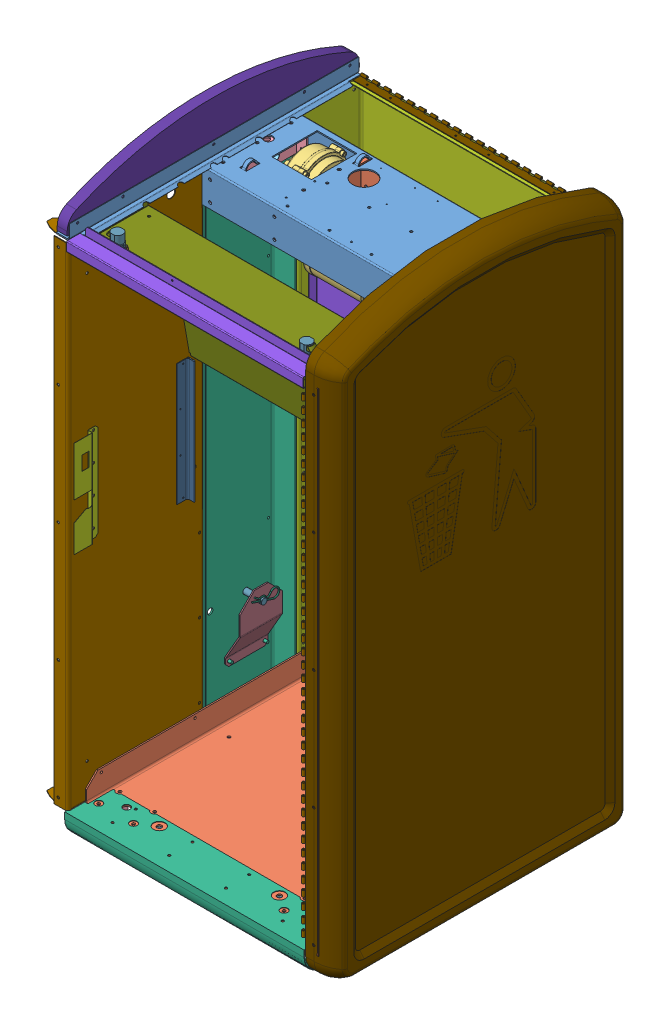
SolidWorks assembly BB3_Chassis, configuration Défaut. Lengths in mm.
Overall size (671.41 1282.03 663.93).
67 component instances, 38 part files, 144 mates.
Components (placement in the parent):
- TopCrossmember_Rev2-1: TopCrossmember_Rev2 [Default] at (20.5473 102.5902 0) size (635 86.99 210.82)
- TopCrossMotorBrkt_Rev3-1: TopCrossMotorBrkt_Rev3 [Défaut] at (-101.9976 61.051 0) size (152.4 200.54 205.51)
- Moto_Reducteur_011_562_1_216-1: Moto_Reducteur_011_562_1_216 [Default] at (192.9322 74.2423 -36.8146) x (0 -0.000019 -1) z (-1 0 0) size (114.3 226.4 239.81)
- TopCrossBearingBrkt_Rev1-1: TopCrossBearingBrkt_Rev1 [Défaut] at (-246.0257 61.051 0) size (25.4 73.66 205.51)
- TopCrossBearingBrkt_Rev1-2: TopCrossBearingBrkt_Rev1 [Défaut] at (287.1203 61.051 0) x (-1 0 0) z (0 0 -1) size (25.4 73.66 205.51)
- Chassis_Coussinet-1: Chassis_Coussinet [Default] at (-247.5497 60.2788 -36.8146) x (0 -0.995993 0.089436) z (0 0.089436 0.995993) size (28.27 19.05 28.27)
- Chassis_Coussinet-2: Chassis_Coussinet [Default] at (288.6443 60.2788 -36.8146) x (0 0.997938 0.064185) z (0 -0.064185 0.997938) size (28.27 19.05 28.27)
- Chassis_Support_Moteur-1: Chassis_Support_Moteur [Défaut] at (-296.9017 100.6288 0.0002) x (0 0 1) z (0 1 0) size (205.51 54 1127)
- Chassis_Support_Moteur-2: Chassis_Support_Moteur [Défaut] at (337.9963 100.6288 0.0002) x (0 0 -1) z (0 1 0) size (205.51 54 1127)
- Chassis_Panneau_Arriere-2: Chassis_Panneau_Arriere [Défaut] at (20.5983 -479.4712 -246.619) x (0 0 1) z (0 1 0) size (164.98 667 1155.29)
- Chassis_Support_Batterie-2: Chassis_Support_Batterie [Défaut] at (20.5983 -270.8192 -242.544) x (0 0 1) z (-1 0 0) size (116.32 446 529)
- Chassis_Support_Moteur_Devant_Gauche-2: Chassis_Support_Moteur_Devant_Gauche [Défaut] at (-249.8894 -442.8187 130.7585) x (0 0 -1) z (0 1 0) size (329.85 66 1105)
- Chassis_Positionnement_Emetteur_Recepteur_Gauche-2: Chassis_Positionnement_Emetteur_Recepteur_Gauche [Défaut] at (-222.4622 -381.8185 156.8606) x (1 0 0) z (0 -1 0) size (22.1 48.5 273)
- Chassis_Support_Moteur_Devant_Droite-1: Chassis_Support_Moteur_Devant_Droite [Défaut] at (290.9839 -442.8187 130.7585) x (0 0 -1) z (0 -1 0) size (329.85 66 1105)
- Chassis_Positionnement_Emetteur_Recepteur_Droite-1: Chassis_Positionnement_Emetteur_Recepteur_Droite [Défaut] at (263.5568 -381.8185 156.8606) x (-1 0 0) z (0 1 0) size (22.1 48.5 273)
- Chassis_Support_Pignon_bas-1: Chassis_Support_Pignon_bas [Défaut] at (305.4963 -865.3715 -39.8528) x (-1 0 0) z (0 0 1) size (35.2 151.29 95)
- Chassis_Axe_Pignon_Bas-1: Chassis_Axe_Pignon_Bas [Défaut] at (340.9963 -816.3715 -39.8528) x (-1 0 0) z (0 -0.052233 -0.998635) size (48.6 15.9 15.9)
- Chassis_Goupille_Axe_Pignon_bas-1: Chassis_Goupille_Axe_Pignon_bas [Défaut] at (300.5463 -817.6251 -63.8201) x (0 0.052233 0.998635) z (1 0 0) size (60.5 23 3)
- Chassis_Support_Pignon_bas-2: Chassis_Support_Pignon_bas [Défaut] at (-264.4017 -865.3715 -39.8528) x (1 0 0) z (0 0 -1) size (35.2 151.29 95)
- Chassis_Axe_Pignon_Bas-2: Chassis_Axe_Pignon_Bas [Défaut] at (-299.9017 -816.3715 -39.8528) x (1 0 0) z (0 0.31653 0.948583) size (48.6 15.9 15.9)
- Chassis_Goupille_Axe_Pignon_bas-2: Chassis_Goupille_Axe_Pignon_bas [Défaut] at (-259.4517 -808.7748 -17.0869) x (0 -0.31653 -0.948583) z (1 0 0) size (60.5 23 3)
- Chassis_Plaque_Haute-1: Chassis_Plaque_Haute [Défaut] at (20.4963 92.768 412.6062) x (0 0 -1) z (1 0 0) size (278.51 354.1 562.7)
- Chassis_Renfort-1: Chassis_Renfort [Défaut] at (20.5463 -1018.8712 0.0002) x (0 0 1) z (-1 0 0) size (199.51 39 641)
- Chassis_Charniere_Photovoltaique-1: Chassis_Charniere_Photovoltaique [Défaut] at (20.5983 134.4053 -220.1468) x (0 0 -1) z (1 0 0) size (21.77 6 520)
- Chassis_Equerre_Haute-1: Chassis_Equerre_Haute [Défaut] at (-246.1446 112.2812 81.6782) x (1 0 0.000001) z (-0.000001 0 1) size (44 37.45 648)
- Chassis_Equerre_Haute-2: Chassis_Equerre_Haute [Défaut] at (287.2893 112.2812 81.6751) x (-1 0 -0.000168) z (0.000168 0 -1) size (44 37.45 648)
- Chassis_Repose_Bac_Dechets-1: Chassis_Repose_Bac_Dechets [Défaut] at (20.4963 -992.8728 80.2436) x (0 -0.000001 1) z (-1 0 0) size (641.73 77 529)
- Chassis_Semelle-1: Chassis_Semelle [Défaut] at (20.4963 -1034.3925 80.4561) x (1 0 0) z (0 -0.000001 1) size (404.15 56 558)
- Chassis_Repose_Pied-1: Chassis_Repose_Pied [Défaut] at (-187.0037 -1049.3185 336.4561) x (1 0 0) z (0 -0.000001 1) size (94 52.5 63.3)
- Chassis_Repose_Pied-2: Chassis_Repose_Pied [Défaut] at (-187.0037 -1049.3182 -175.5439) x (1 0 0) z (0 -0.000001 1) size (94 52.5 63.3)
- Chassis_Repose_Pied-3: Chassis_Repose_Pied [Défaut] at (227.9963 -1049.3182 -175.5439) x (1 0 0) z (0 -0.000001 1) size (94 52.5 63.3)
- Chassis_Repose_Pied-4: Chassis_Repose_Pied [Défaut] at (227.9963 -1049.3185 336.4561) x (1 0 0) z (0 -0.000001 1) size (94 52.5 63.3)
- Chassis_Repose_Pied_Insert-1: Chassis_Repose_Pied_Insert [Défaut] at (-187.0037 -1050.3185 336.4561) x (0 1 0.000001) z (0.428959 -0.000001 0.903324) size (14.3 17.5 17.5)
- Chassis_Repose_Pied_Insert-2: Chassis_Repose_Pied_Insert [Défaut] at (227.9963 -1050.3185 336.4561) x (0 1 0.000001) z (0.384049 -0.000001 0.923313) size (14.3 17.5 17.5)
- Chassis_Repose_Pied_Insert-3: Chassis_Repose_Pied_Insert [Défaut] at (227.9963 -1050.3182 -175.5439) x (0 1 0.000001) z (-0.000001 -0.000001 1) size (14.3 17.5 17.5)
- Chassis_Repose_Pied_Insert-4: Chassis_Repose_Pied_Insert [Défaut] at (-187.0037 -1050.3182 -175.5439) x (0 1 0.000001) z (-0.000001 -0.000001 1) size (14.3 17.5 17.5)
- Chassis_Repose_Pied_Insert-5: Chassis_Repose_Pied_Insert [Défaut] at (-114.0037 -995.8185 336.4561) x (0 -1 -0.000001) z (0.798225 0 0.602359) size (14.3 17.5 17.5)
- Chassis_Repose_Pied_Insert-6: Chassis_Repose_Pied_Insert [Défaut] at (154.9963 -995.8185 336.4561) x (0 -1 -0.000001) z (0.000001 -0.000001 1) size (14.3 17.5 17.5)
- Chassis_Repose_Pied_Insert-7: Chassis_Repose_Pied_Insert [Défaut] at (-114.0037 -995.8182 -175.5439) x (0 -1 -0.000001) z (0.000001 -0.000001 1) size (14.3 17.5 17.5)
- Chassis_Repose_Pied_Insert-8: Chassis_Repose_Pied_Insert [Défaut] at (154.9963 -995.8182 -175.5439) x (0 -1 -0.000001) z (0.000001 -0.000001 1) size (14.3 17.5 17.5)
- Chassis_Dessous_Avant_Porte-1: Chassis_Dessous_Avant_Porte [Défaut] at (20.4963 -992.8728 80.2436) x (0 -0.000001 1) z (-1 0 0) size (98 53.79 536)
- Chassis_Serrure-1: Chassis_Serrure [Défaut] at (-243.4017 -382.964 366.4072) x (1 0 0) z (0 1 0) size (10.5 63.82 216)
- Chassis_Equerre_Face-1: Chassis_Equerre_Face [Défaut] at (20.4963 111.0096 411.9878) x (0 0 1) z (-1 0 0) size (32.2 41.42 529)
- Chassis_Charniere_Support_Moteur_Devant_Droite-1: Chassis_Charniere_Support_Moteur_Devant_Droite [Défaut] at (260.2718 -465.3185 388.412) x (0 0 1) z (0 -1 0) size (21.77 6 1066)
- Chassis_Serrure_Cle-1: Chassis_Serrure_Cle [Défaut] at (-191.3537 126.1269 363.7894) x (0 1 0) z (-1 0 0) size (41.58 38.56 38.97)
  - Chassis_Serrure_Came-1: Chassis_Serrure_Came [Défaut] at (-18.246 14.5659 16.3878) x (0 -1 0) z (1 0 0) size (12.45 12.01 13.54)
  - Chassis_Serrure_Rondelle_Ecrou-1: Chassis_Serrure_Rondelle_Ecrou [Défaut] at (-31.074 17.7899 -9.8703) x (0 0.096744 0.995309) z (-1 0 0) size (35.31 35.31 0.64)
  - Chassis_Serrure_Ecrou_Hex-1: Chassis_Serrure_Ecrou_Hex [Défaut] at (-26.3115 -31.157 8.2014) x (0 0 1) z (-1 0 0) size (33 28.58 4.76)
  - Chassis_Serrure_Insert_Cle-1: Chassis_Serrure_Insert_Cle [Défaut] at (26.379 -212.8643 14.6) x (-1 0 0) z (0 0 -1) size (23.33 15.95 15.95)
  - Chassis_Serrure_Support-1: Chassis_Serrure_Support [Défaut] at (-26.6815 11.1833 12.473) x (-1 0 0) z (0 -1 0) size (41.46 28.7 28.7)
  - Chassis_Serrure_Ressort-1: Chassis_Serrure_Ressort [Défaut] at (-1.4058 10.243 9.1044) x (0 0 -1) z (1 0 0) size (21.49 4.59 4.57)
  - Chassis_Serrure_Pene-1: Chassis_Serrure_Pene [Défaut] at (1.0072 5.2825 -10.1896) x (0 -0.999973 -0.007317) z (-1 0 0) size (16.91 23.47 9.63)
- Chassis_Serrure_Cle-2: Chassis_Serrure_Cle [Défaut] at (232.3463 126.1269 341.4229) x (0 1 0) z (1 0 0) size (41.58 38.56 38.97)
  - Chassis_Serrure_Came-1: Chassis_Serrure_Came [Défaut] at (-18.246 14.5659 16.3878) x (0 -1 0) z (1 0 0) size (12.45 12.01 13.54)
  - Chassis_Serrure_Rondelle_Ecrou-1: Chassis_Serrure_Rondelle_Ecrou [Défaut] at (-31.074 17.7899 -9.8703) x (0 0.096744 0.995309) z (-1 0 0) size (35.31 35.31 0.64)
  - Chassis_Serrure_Ecrou_Hex-1: Chassis_Serrure_Ecrou_Hex [Défaut] at (-26.3115 -31.157 8.2014) x (0 0 1) z (-1 0 0) size (33 28.58 4.76)
  - Chassis_Serrure_Insert_Cle-1: Chassis_Serrure_Insert_Cle [Défaut] at (26.379 -212.8643 14.6) x (-1 0 0) z (0 0 -1) size (23.33 15.95 15.95)
  - Chassis_Serrure_Support-1: Chassis_Serrure_Support [Défaut] at (-26.6815 11.1833 12.473) x (-1 0 0) z (0 -1 0) size (41.46 28.7 28.7)
  - Chassis_Serrure_Ressort-1: Chassis_Serrure_Ressort [Défaut] at (-1.4058 10.243 9.1044) x (0 0 -1) z (1 0 0) size (21.49 4.59 4.57)
  - Chassis_Serrure_Pene-1: Chassis_Serrure_Pene [Défaut] at (1.0072 5.2825 -10.1896) x (0 -0.999973 -0.007317) z (-1 0 0) size (16.91 23.47 9.63)
- Tombstone_Rev1-1: Tombstone_Rev1 [Default] at (288.5894 129.5652 81.0473) x (1 0 0.000168) z (-0.000168 0 1) size (22.23 105.62 654.05)
- Tombstone_Rev1-2: Tombstone_Rev1 [Default] at (-247.4446 129.5652 82.3062) x (-1 0 -0.000001) z (0.000001 0 -1) size (22.23 105.62 654.05)
- SideSkin_Rev1-1: SideSkin_Rev1 [Default] at (-317.3073 -1045.6118 82.3061) x (-1 0 -0.000001) z (0.000001 0 -1) size (69.87 1274.83 660.4) (hidden)
- SideSkin_Rev1-2: SideSkin_Rev1 [Default] at (358.4521 -1045.6118 81.059) x (1 0 0.000168) z (-0.000168 0 1) size (69.87 1274.83 660.4)
- Chassis_Interieur_Cache_Chaine-1: Chassis_Interieur_Cache_Chaine [Défaut] at (-242.9017 -763.8184 0) x (0 -0.000001 1) z (-1 0 0) size (249 989 21) (hidden)
- Chassis_Interieur_Cache_Chaine-2: Chassis_Interieur_Cache_Chaine [Défaut] at (283.9963 -763.8185 0.0002) x (0 0 -1) z (1 0 0) size (249 989 21)
- Chassis_Bac_Dechets-1: Chassis_Bac_Dechets [Défaut] at (19.5983 -711.9931 65.1059) x (-1 0 0) z (0 0.000001 -1) size (517 387.96 620.45) (hidden)
Mates (geometry in assembly coordinates):
- Coïncidente2: coincident anti-aligned: plane of TopCrossmember_Rev2-1 through (338.0473 102.5902 -102.7532) normal (0 0 1); plane of TopCrossMotorBrkt_Rev3-1 through (50.4024 28.92 -102.7532) normal (0 0 -1)
- Coaxiale4: concentric aligned: cylinder of TopCrossmember_Rev2-1 through (-87.4027 86.197 105.41) axis (0 0 1) radius 3.3735; cylinder of TopCrossMotorBrkt_Rev3-1 through (-87.4027 86.197 102.7532) axis (0 0 1) radius 3.3735
- Coaxiale5: concentric aligned: cylinder of TopCrossmember_Rev2-1 through (-87.4027 41.747 105.41) axis (0 0 1) radius 3.3735; cylinder of TopCrossMotorBrkt_Rev3-1 through (-87.4027 41.747 102.7532) axis (0 0 1) radius 3.3735
- Coïncidente3: coincident anti-aligned: plane of TopCrossMotorBrkt_Rev3-1 through (-101.9976 19.522 -102.7532) normal (-1 0 0); plane of Moto_Reducteur_011_562_1_216-1 through (-101.9976 60.2791 -36.8143) normal (1 0 0)
- Coaxiale6: concentric anti-aligned: cylinder of TopCrossMotorBrkt_Rev3-1 through (-99.3407 60.2788 -36.8146) axis (-1 0 0) radius 15.24; cylinder of Moto_Reducteur_011_562_1_216-1 through (-181.2456 60.2791 -36.8143) axis (1 0 0) radius 9.525
- Coaxiale7: concentric anti-aligned: cylinder of TopCrossMotorBrkt_Rev3-1 through (-99.3407 33.3368 -63.7556) axis (-1 0 0) radius 3.683; cylinder of Moto_Reducteur_011_562_1_216-1 through (-101.9976 33.3368 -63.7556) axis (1 0 0) radius 3.175
- Coïncidente4: coincident anti-aligned: plane of TopCrossmember_Rev2-1 through (-296.9527 102.5902 102.7532) normal (0 0 -1); plane of TopCrossBearingBrkt_Rev1-1 through (-243.3689 94.96 102.7532) normal (0 0 1)
- Coaxiale8: concentric aligned: cylinder of TopCrossmember_Rev2-1 through (-231.4207 86.197 105.41) axis (0 0 1) radius 3.3735; cylinder of TopCrossBearingBrkt_Rev1-1 through (-231.4207 86.197 102.7532) axis (0 0 1) radius 3.3735
- Coaxiale9: concentric aligned: cylinder of TopCrossmember_Rev2-1 through (-231.4207 41.747 105.41) axis (0 0 1) radius 3.3735; cylinder of TopCrossBearingBrkt_Rev1-1 through (-231.4207 41.747 102.7532) axis (0 0 1) radius 3.3735
- Coïncidente5: coincident anti-aligned: plane of TopCrossmember_Rev2-1 through (338.0473 102.5902 -102.7532) normal (0 0 1); plane of TopCrossBearingBrkt_Rev1-2 through (284.4634 94.96 -102.7532) normal (0 0 -1)
- Coaxiale10: concentric anti-aligned: cylinder of TopCrossmember_Rev2-1 through (272.5153 86.197 105.41) axis (0 0 1) radius 3.3735; cylinder of TopCrossBearingBrkt_Rev1-2 through (272.5153 86.197 -102.7532) axis (0 0 -1) radius 3.3735
- Coaxiale11: concentric anti-aligned: cylinder of TopCrossmember_Rev2-1 through (272.5153 41.747 105.41) axis (0 0 1) radius 3.3735; cylinder of TopCrossBearingBrkt_Rev1-2 through (272.5153 41.747 -102.7532) axis (0 0 -1) radius 3.3735
- Coïncidente6: coincident anti-aligned: plane of TopCrossBearingBrkt_Rev1-1 through (-246.0257 19.522 -102.7532) normal (-1 0 0); plane of Chassis_Coussinet-1 through (-246.0257 60.2788 -36.8146) normal (1 0 0)
- Coaxiale12: concentric anti-aligned: cylinder of TopCrossBearingBrkt_Rev1-1 through (-243.3689 60.2788 -36.8146) axis (-1 0 0) radius 11.1125; cylinder of Chassis_Coussinet-1 through (-247.5497 60.2788 -36.8146) axis (1 0 0) radius 9.6139
- Coaxiale13: concentric anti-aligned: cylinder of TopCrossBearingBrkt_Rev1-2 through (284.4634 60.2788 -36.8146) axis (1 0 0) radius 11.1125; cylinder of Chassis_Coussinet-2 through (269.5943 60.2788 -36.8146) axis (-1 0 0) radius 11.1125
- Coïncidente7: coincident anti-aligned: plane of TopCrossBearingBrkt_Rev1-2 through (287.1203 19.522 102.7532) normal (1 0 0); plane of Chassis_Coussinet-2 through (287.1203 60.2788 -36.8146) normal (-1 0 0)
- Coïncidente8: coincident anti-aligned: plane of TopCrossmember_Rev2-1 through (-269.9017 102.5902 0) normal (-1 0 0); plane of Chassis_Support_Moteur-1
- Coïncidente12: coincident anti-aligned: plane of TopCrossmember_Rev2-1 through (-296.9527 102.5902 102.7532) normal (0 0 -1); plane of Chassis_Support_Moteur-1 through (-299.9017 100.6288 102.7532) normal (0 0 1)
- Coïncidente13: coincident anti-aligned: plane of TopCrossBearingBrkt_Rev1-1 through (-246.0257 60.2788 0) normal (0 1 0); plane of Chassis_Support_Moteur-1
- Coïncidente14: coincident anti-aligned: plane of TopCrossmember_Rev2-1 through (-296.9527 102.5902 102.7532) normal (0 0 -1); plane of Chassis_Support_Moteur-2 through (286.9963 100.6288 102.7532) normal (0 0 1)
- Coïncidente15: coincident anti-aligned: plane of TopCrossBearingBrkt_Rev1-2; plane of Chassis_Support_Moteur-2
- Coïncidente16: coincident anti-aligned: plane of TopCrossmember_Rev2-1 through (310.9963 102.5902 0) normal (1 0 0); plane of Chassis_Support_Moteur-2
- Coaxiale15: concentric aligned: cylinder of Chassis_Support_Moteur-1 through (-298.4017 10.6288 -90.7528) axis (1 0 0) radius 2.45; cylinder of Chassis_Panneau_Arriere-2 through (-301.4017 10.6288 -90.7528) axis (1 0 0) radius 2.7
- Coaxiale16: concentric aligned: cylinder of Chassis_Support_Moteur-1 through (-298.4017 -903.3712 -90.7528) axis (1 0 0) radius 2.45; cylinder of Chassis_Panneau_Arriere-2 through (-301.4017 -903.3712 -90.7528) axis (1 0 0) radius 2.7
- Coïncidente19: coincident anti-aligned: plane of Chassis_Support_Moteur-1 through (-299.9017 100.6288 0.0002) normal (-1 0 0); plane of Chassis_Panneau_Arriere-2 through (-299.9017 -1095.4712 -106.044) normal (1 0 0)
- Coïncidente20: coincident anti-aligned: plane of Chassis_Panneau_Arriere-2 through (285.0983 -998.3712 -112.044) normal (-1 0 0); plane of Chassis_Support_Batterie-2 through (285.0983 -476.3192 -146.144) normal (1 0 0)
- Coaxiale17: concentric aligned: cylinder of Chassis_Panneau_Arriere-2 through (285.8483 -484.8192 -214.144) axis (-1 0 0) radius 2.7; cylinder of Chassis_Support_Batterie-2 through (285.0983 -484.8192 -214.144) axis (-1 0 0) radius 2.7
- Coaxiale18: concentric aligned: cylinder of Chassis_Panneau_Arriere-2 through (285.8483 -484.8192 -158.144) axis (-1 0 0) radius 2.7; cylinder of Chassis_Support_Batterie-2 through (285.0983 -484.8192 -158.144) axis (-1 0 0) radius 2.7
- Coaxiale19: concentric aligned: cylinder of Chassis_Support_Moteur-1 through (-299.9017 10.6288 90.7532) axis (1 0 0) radius 2.45; cylinder of Chassis_Support_Moteur_Devant_Gauche-2 through (-301.4017 10.6288 90.7532) axis (1 0 0) radius 2.7
- Coaxiale20: concentric aligned: cylinder of Chassis_Support_Moteur-1 through (-299.9017 -903.3712 90.7532) axis (1 0 0) radius 2.45; cylinder of Chassis_Support_Moteur_Devant_Gauche-2 through (-301.4017 -903.3712 90.7532) axis (1 0 0) radius 2.7
- Coïncidente21: coincident anti-aligned: plane of Chassis_Support_Moteur-1 through (-299.9017 100.6288 0.0002) normal (-1 0 0); plane of Chassis_Support_Moteur_Devant_Gauche-2 through (-299.9017 -1056.8712 80.7532) normal (1 0 0)
- Coïncidente22: coincident anti-aligned: plane of Chassis_Support_Moteur_Devant_Gauche-2 through (-243.9017 -1056.8712 104.9532) normal (1 0 0); plane of Chassis_Positionnement_Emetteur_Recepteur_Gauche-2 through (-243.9017 -245.3185 143.1532) normal (-1 0 0)
- Coaxiale21: concentric aligned: cylinder of Chassis_Support_Moteur_Devant_Gauche-2 through (-245.4017 -426.8185 160.4532) axis (1 0 0) radius 1.5; cylinder of Chassis_Positionnement_Emetteur_Recepteur_Gauche-2 through (-243.9017 -426.8185 160.4532) axis (1 0 0) radius 1.5
- Coaxiale22: concentric aligned: cylinder of Chassis_Support_Moteur_Devant_Gauche-2 through (-245.4017 -336.8185 160.4532) axis (1 0 0) radius 1.5; cylinder of Chassis_Positionnement_Emetteur_Recepteur_Gauche-2 through (-243.9017 -336.8185 160.4532) axis (1 0 0) radius 1.5
- Coïncidente24: coincident anti-aligned: plane of Chassis_Support_Moteur-2 through (340.9963 100.6288 0.0002) normal (1 0 0); plane of Chassis_Support_Moteur_Devant_Droite-1 through (340.9963 27.0338 80.7532) normal (-1 0 0)
- Coaxiale25: concentric aligned: cylinder of Chassis_Support_Moteur-2 through (339.4963 10.6288 90.7532) axis (-1 0 0) radius 2.45; cylinder of Chassis_Support_Moteur_Devant_Droite-1 through (341.7463 10.6288 90.7532) axis (-1 0 0) radius 2.7
- Coaxiale26: concentric aligned: cylinder of Chassis_Support_Moteur-2 through (339.4963 -903.3712 90.7532) axis (-1 0 0) radius 2.45; cylinder of Chassis_Support_Moteur_Devant_Droite-1 through (341.7463 -903.3712 90.7532) axis (-1 0 0) radius 2.7
- Coïncidente26: coincident anti-aligned: plane of Chassis_Support_Moteur_Devant_Droite-1 through (284.9963 103.6812 110.9532) normal (-1 0 0); plane of Chassis_Positionnement_Emetteur_Recepteur_Droite-1 through (284.9963 -245.3185 168.4532) normal (1 0 0)
- Coaxiale27: concentric aligned: cylinder of Chassis_Support_Moteur_Devant_Droite-1 through (285.7463 -336.8185 160.4532) axis (-1 0 0) radius 1.5; cylinder of Chassis_Positionnement_Emetteur_Recepteur_Droite-1 through (284.3463 -336.8185 160.4532) axis (-1 0 0) radius 1.5
- Coaxiale28: concentric aligned: cylinder of Chassis_Support_Moteur_Devant_Droite-1 through (285.7463 -426.8185 160.4532) axis (-1 0 0) radius 1.5; cylinder of Chassis_Positionnement_Emetteur_Recepteur_Droite-1 through (284.3463 -426.8185 160.4532) axis (-1 0 0) radius 1.5
- Coïncidente27: coincident anti-aligned: plane of Chassis_Support_Moteur-2 through (337.9963 100.6288 -99.7528) normal (-1 0 0); plane of Chassis_Support_Pignon_bas-1 through (337.9963 -921.6632 -87.3528) normal (1 0 0)
- Coaxiale29: concentric aligned: cylinder of Chassis_Support_Moteur-2 through (340.9963 -930.8712 -79.7058) axis (-1 0 0) radius 3; cylinder of Chassis_Support_Pignon_bas-1 through (337.9963 -930.8712 -79.7058) axis (-1 0 0) radius 3.5
- Coaxiale30: concentric aligned: cylinder of Chassis_Support_Moteur-2 through (340.9963 -930.8712 0.0002) axis (-1 0 0) radius 3; cylinder of Chassis_Support_Pignon_bas-1 through (337.9963 -930.8712 0.0002) axis (-1 0 0) radius 3.5
- Coïncidente28: coincident anti-aligned: plane of Chassis_Support_Moteur-2 through (340.9963 100.6288 0.0002) normal (1 0 0); plane of Chassis_Axe_Pignon_Bas-1 through (340.9963 -812.4019 -40.0605) normal (-1 0 0)
- Coaxiale31: concentric anti-aligned: cylinder of Chassis_Support_Pignon_bas-1 through (302.7963 -816.3715 -39.8528) axis (1 0 0) radius 6.5; cylinder of Chassis_Axe_Pignon_Bas-1 through (318.6963 -816.3715 -39.8528) axis (-1 0 0) radius 6.25
- Coaxiale32: concentric anti-aligned: cylinder of Chassis_Axe_Pignon_Bas-1 through (300.5463 -819.1686 -93.3295) axis (0 -0.052233 -0.998635) radius 2.15; cylinder of Chassis_Goupille_Axe_Pignon_bas-1 through (300.5463 -817.6251 -63.8201) axis (0 0.052233 0.998635) radius 1.5
- Parallèle1: parallel anti-aligned: plane of Chassis_Support_Pignon_bas-1 through (302.7963 -866.095 -87.3528) normal (-1 0 0); plane of Chassis_Goupille_Axe_Pignon_bas-1 through (300.5463 -817.6251 -63.8201) normal (1 0 0)
- Tangent2: tangent: cylinder of Chassis_Axe_Pignon_Bas-1 through (318.6963 -816.3715 -39.8528) axis (-1 0 0) radius 6.25; face of Chassis_Goupille_Axe_Pignon_bas-1
- Coïncidente29: coincident anti-aligned: plane of Chassis_Support_Moteur-1 through (-296.9017 100.6288 99.7532) normal (1 0 0); plane of Chassis_Support_Pignon_bas-2 through (-296.9017 -913.016 6.2972) normal (-1 0 0)
- Coaxiale33: concentric aligned: cylinder of Chassis_Support_Moteur-1 through (-296.9017 -930.8712 -79.7058) axis (1 0 0) radius 3; cylinder of Chassis_Support_Pignon_bas-2 through (-296.9017 -930.8712 -79.7058) axis (1 0 0) radius 3.5
- Coïncidente30: coincident anti-aligned: plane of Chassis_Support_Moteur-1 through (-299.9017 100.6288 0.0002) normal (-1 0 0); plane of Chassis_Axe_Pignon_Bas-2 through (-299.9017 -809.2033 -52.7033) normal (1 0 0)
- Coaxiale35: concentric anti-aligned: cylinder of Chassis_Support_Pignon_bas-2 through (-261.7017 -812.9739 -51.4451) axis (-1 0 0) radius 6.5; cylinder of Chassis_Axe_Pignon_Bas-2 through (-277.6017 -812.9739 -51.4451) axis (1 0 0) radius 6.25
- Coaxiale36: concentric anti-aligned: cylinder of Chassis_Axe_Pignon_Bas-2 through (-259.4517 -796.0238 -0.6487) axis (0 0.31653 0.948583) radius 2.15; cylinder of Chassis_Goupille_Axe_Pignon_bas-2 through (-259.4517 -805.3772 -28.6791) axis (0 -0.31653 -0.948583) radius 1.5
- Parallèle2: parallel aligned: plane of Chassis_Support_Pignon_bas-2 through (-261.7017 -857.7236 0.7674) normal (1 0 0); plane of Chassis_Goupille_Axe_Pignon_bas-2 through (-259.4517 -805.3772 -28.6791) normal (1 0 0)
- Tangent3: tangent: cylinder of Chassis_Axe_Pignon_Bas-2 through (-277.6017 -812.9739 -51.4451) axis (1 0 0) radius 6.25; face of Chassis_Goupille_Axe_Pignon_bas-2
- Coaxiale39: concentric aligned: cylinder of Chassis_Support_Moteur_Devant_Droite-1 through (285.7463 99.9922 260.6062) axis (-1 0 0) radius 2.7; cylinder of Chassis_Plaque_Haute-1 through (284.1713 99.9922 260.6062) axis (-1 0 0) radius 2.7
- Coaxiale40: concentric aligned: cylinder of Chassis_Support_Moteur_Devant_Droite-1 through (285.7463 99.9922 387.6062) axis (-1 0 0) radius 2.7; cylinder of Chassis_Plaque_Haute-1 through (284.1713 99.9922 387.6062) axis (-1 0 0) radius 2.7
- Coïncidente32: coincident anti-aligned: plane of Chassis_Support_Moteur_Devant_Droite-1 through (284.9963 103.6812 110.9532) normal (-1 0 0); plane of Chassis_Plaque_Haute-1 through (284.9963 -169.3578 412.6062) normal (1 0 0)
- Coaxiale41: concentric anti-aligned: cylinder of Chassis_Support_Moteur-2 through (314.9963 -1012.3712 -102.7528) axis (0 0 1) radius 5; cylinder of Chassis_Renfort-1 through (314.9963 -1012.3712 -96.7528) axis (0 0 -1) radius 4.25
- Coïncidente33: coincident anti-aligned: plane of Chassis_Support_Moteur-2 through (286.9963 100.6288 -99.7528) normal (0 0 1); plane of Chassis_Renfort-1 through (341.0463 -1038.3712 -99.7528) normal (0 0 -1)
- Angle1: planar angle = 0 rad aligned: plane of Chassis_Support_Moteur-2 through (330.2237 -1026.3712 -67.6038) normal (0 -1 0); plane of Chassis_Renfort-1 through (341.0463 -1002.3712 96.7532) normal (0 -1 0)
- Coïncidente34: coincident anti-aligned: plane of Chassis_Panneau_Arriere-2 through (-245.4017 109.6808 -1447.8763) normal (0 1 0); plane of Chassis_Charniere_Photovoltaique-1 through (20.5983 109.6808 -241.391) normal (0 -1 0)
- Coaxiale42: concentric anti-aligned: cylinder of Chassis_Panneau_Arriere-2 through (255.5983 109.6808 -229.619) axis (0 -1 0) radius 2.7; cylinder of Chassis_Charniere_Photovoltaique-1 through (255.5983 109.6808 -229.619) axis (0 1 0) radius 1.75
- Coaxiale43: concentric anti-aligned: cylinder of Chassis_Panneau_Arriere-2 through (-214.4017 109.6808 -229.619) axis (0 -1 0) radius 2.7; cylinder of Chassis_Charniere_Photovoltaique-1 through (-214.4017 109.6808 -229.619) axis (0 1 0) radius 1.75
- Coïncidente35: coincident anti-aligned: plane of Chassis_Support_Moteur_Devant_Gauche-2 through (918.7559 109.6812 104.9532) normal (0 1 0); plane of Chassis_Equerre_Haute-1 through (-241.0792 109.6812 81.6782) normal (0 -1 0)
- Coaxiale46: concentric anti-aligned: cylinder of Chassis_Support_Moteur_Devant_Gauche-2 through (-264.6447 108.9312 379.9532) axis (0 -1 0) radius 2.7; cylinder of Chassis_Equerre_Haute-1 through (-264.6447 110.9812 379.9532) axis (0 1 0) radius 2.85
- Coaxiale47: concentric anti-aligned: cylinder of Chassis_Panneau_Arriere-2 through (-264.6444 109.6808 -226.322) axis (0 -1 0) radius 2.6; cylinder of Chassis_Equerre_Haute-1 through (-264.6444 110.9812 -226.3218) axis (0 1 0) radius 2.85
- Coïncidente38: coincident anti-aligned: plane of Chassis_Support_Moteur_Devant_Droite-1 through (350.9966 109.6812 110.9532) normal (0 1 0); plane of Chassis_Equerre_Haute-2 through (282.224 109.6812 81.6742) normal (0 -1 0)
- Coaxiale48: concentric anti-aligned: cylinder of Chassis_Support_Moteur_Devant_Droite-1 through (305.7393 109.6812 379.9532) axis (0 -1 0) radius 2.7; cylinder of Chassis_Equerre_Haute-2 through (305.7393 110.9812 379.9532) axis (0 1 0) radius 2.85
- Coaxiale49: concentric anti-aligned: cylinder of Chassis_Panneau_Arriere-2 through (305.841 108.9308 -226.322) axis (0 -1 0) radius 2.6; cylinder of Chassis_Equerre_Haute-2 through (305.841 110.9812 -226.3218) axis (0 1 0) radius 2.85
- Coaxiale50: concentric aligned: cylinder of Chassis_Panneau_Arriere-2 through (285.8483 -950.8182 -172.627) axis (-1 0 0) radius 2.7; cylinder of Chassis_Repose_Bac_Dechets-1 through (284.9963 -950.8182 -172.6268) axis (-1 0 0) radius 2.7
- Coaxiale51: concentric aligned: cylinder of Chassis_Support_Moteur_Devant_Droite-1 through (285.7463 -950.8185 339.1062) axis (-1 0 0) radius 2.7; cylinder of Chassis_Repose_Bac_Dechets-1 through (284.9963 -950.8185 339.1062) axis (-1 0 0) radius 2.7
- Coïncidente39: coincident anti-aligned: plane of Chassis_Support_Moteur_Devant_Droite-1 through (284.9963 103.6812 110.9532) normal (-1 0 0); plane of Chassis_Repose_Bac_Dechets-1 through (284.9963 -968.3183 80.2436) normal (1 0 0)
- Coïncidente40: coincident anti-aligned: plane of Chassis_Repose_Bac_Dechets-1 through (284.9963 -996.8185 398.1061) normal (0 -1 -0.000001); plane of Chassis_Semelle-1 through (-128.6584 -996.8181 -198.5439) normal (0 1 0.000001)
- Coaxiale53: concentric aligned: cylinder of Chassis_Repose_Bac_Dechets-1 through (-114.0037 -993.8185 336.4561) axis (0 -1 -0.000001) radius 5.25; cylinder of Chassis_Semelle-1 through (-114.0037 -996.8185 336.4561) axis (0 -1 -0.000001) radius 6.75
- Coaxiale54: concentric aligned: cylinder of Chassis_Repose_Bac_Dechets-1 through (-114.0037 -993.8182 -175.5439) axis (0 -1 -0.000001) radius 5.25; cylinder of Chassis_Semelle-1 through (-114.0037 -996.8182 -175.5439) axis (0 -1 -0.000001) radius 6.75
- Coïncidente41: coincident anti-aligned: plane of Chassis_Repose_Bac_Dechets-1 through (284.9963 -996.8185 398.1061) normal (0 -1 -0.000001); plane of Chassis_Repose_Pied-1 through (-234.0037 -996.8185 304.8061) normal (0 1 0.000001)
- Coaxiale55: concentric aligned: cylinder of Chassis_Repose_Bac_Dechets-1 through (-226.0037 -993.8185 312.8061) axis (0 -1 -0.000001) radius 3.25; cylinder of Chassis_Repose_Pied-1 through (-226.0037 -996.8185 312.8061) axis (0 -1 -0.000001) radius 3.25
- Coaxiale56: concentric aligned: cylinder of Chassis_Repose_Bac_Dechets-1 through (-226.0037 -993.8185 360.1061) axis (0 -1 -0.000001) radius 3.25; cylinder of Chassis_Repose_Pied-1 through (-226.0037 -996.8185 360.1061) axis (0 -1 -0.000001) radius 3.25
- Coïncidente42: coincident anti-aligned: plane of Chassis_Repose_Bac_Dechets-1 through (284.9963 -996.8185 398.1061) normal (0 -1 -0.000001); plane of Chassis_Repose_Pied-2 through (-234.0037 -996.8181 -207.1939) normal (0 1 0.000001)
- Coaxiale57: concentric aligned: cylinder of Chassis_Repose_Bac_Dechets-1 through (-226.0037 -993.8182 -151.8939) axis (0 -1 -0.000001) radius 3.25; cylinder of Chassis_Repose_Pied-2 through (-226.0037 -996.8182 -151.8939) axis (0 -1 -0.000001) radius 3.25
- Coaxiale58: concentric aligned: cylinder of Chassis_Repose_Bac_Dechets-1 through (-226.0037 -993.8181 -199.1939) axis (0 -1 -0.000001) radius 3.25; cylinder of Chassis_Repose_Pied-2 through (-226.0037 -996.8181 -199.1939) axis (0 -1 -0.000001) radius 3.25
- Coïncidente43: coincident anti-aligned: plane of Chassis_Repose_Bac_Dechets-1 through (284.9963 -996.8185 398.1061) normal (0 -1 -0.000001); plane of Chassis_Repose_Pied-3 through (180.9963 -996.8181 -207.1939) normal (0 1 0.000001)
- Coaxiale59: concentric aligned: cylinder of Chassis_Repose_Bac_Dechets-1 through (188.9963 -993.8181 -199.1939) axis (0 -1 -0.000001) radius 3.25; cylinder of Chassis_Repose_Pied-3 through (188.9963 -996.8181 -199.1939) axis (0 -1 -0.000001) radius 3.25
- Coaxiale60: concentric aligned: cylinder of Chassis_Repose_Bac_Dechets-1 through (266.9963 -993.8182 -151.8939) axis (0 -1 -0.000001) radius 3.25; cylinder of Chassis_Repose_Pied-3 through (266.9963 -998.0682 -151.8939) axis (0 -1 -0.000001) radius 3.25
- Coïncidente44: coincident anti-aligned: plane of Chassis_Repose_Bac_Dechets-1 through (284.9963 -996.8185 398.1061) normal (0 -1 -0.000001); plane of Chassis_Repose_Pied-4 through (262.9963 -996.8185 304.8061) normal (0 1 0.000001)
- Coaxiale61: concentric aligned: cylinder of Chassis_Repose_Bac_Dechets-1 through (266.9963 -993.8185 312.8061) axis (0 -1 -0.000001) radius 3.25; cylinder of Chassis_Repose_Pied-4 through (266.9963 -998.0685 312.8061) axis (0 -1 -0.000001) radius 3.25
- Coaxiale62: concentric aligned: cylinder of Chassis_Repose_Bac_Dechets-1 through (266.9963 -993.8185 360.1061) axis (0 -1 -0.000001) radius 3.25; cylinder of Chassis_Repose_Pied-4 through (266.9963 -998.0685 360.1061) axis (0 -1 -0.000001) radius 3.25
- Coïncidente46: coincident anti-aligned: plane of Chassis_Repose_Pied-4 through (227.9963 -1049.3185 304.8061) normal (0 -1 -0.000001); plane of Chassis_Repose_Pied_Insert-2 through (220.8406 -1049.3185 339.4325) normal (0 1 0.000001)
- Coaxiale63: concentric anti-aligned: cylinder of Chassis_Repose_Pied-4 through (227.9963 -1046.8185 336.4561) axis (0 -1 -0.000001) radius 6.75; cylinder of Chassis_Repose_Pied_Insert-2 through (227.9963 -1040.4185 336.4561) axis (0 1 0.000001) radius 6.75
- Coïncidente47: coincident anti-aligned: plane of Chassis_Repose_Pied-1 through (-187.0037 -1049.3185 304.8061) normal (0 -1 -0.000001); plane of Chassis_Repose_Pied_Insert-1 through (-194.0045 -1049.3185 339.7805) normal (0 1 0.000001)
- Coaxiale64: concentric anti-aligned: cylinder of Chassis_Repose_Pied-1 through (-187.0037 -1046.8185 336.4561) axis (0 -1 -0.000001) radius 6.75; cylinder of Chassis_Repose_Pied_Insert-1 through (-187.0037 -1040.4185 336.4561) axis (0 1 0.000001) radius 6.75
- Coïncidente48: coincident anti-aligned: plane of Chassis_Repose_Pied-3 through (227.9963 -1049.3181 -207.1939) normal (0 -1 -0.000001); plane of Chassis_Repose_Pied_Insert-3 through (220.2463 -1049.3182 -175.5439) normal (0 1 0.000001)
- Coaxiale65: concentric anti-aligned: cylinder of Chassis_Repose_Pied-3 through (227.9963 -1046.8182 -175.5439) axis (0 -1 -0.000001) radius 6.75; cylinder of Chassis_Repose_Pied_Insert-3 through (227.9963 -1040.4182 -175.5439) axis (0 1 0.000001) radius 6.75
- Coïncidente49: coincident anti-aligned: plane of Chassis_Repose_Pied-2 through (-187.0037 -1049.3181 -207.1939) normal (0 -1 -0.000001); plane of Chassis_Repose_Pied_Insert-4 through (-194.7537 -1049.3182 -175.5439) normal (0 1 0.000001)
- Coaxiale66: concentric anti-aligned: cylinder of Chassis_Repose_Pied-2 through (-187.0037 -1046.8182 -175.5439) axis (0 -1 -0.000001) radius 6.75; cylinder of Chassis_Repose_Pied_Insert-4 through (-187.0037 -1040.4182 -175.5439) axis (0 1 0.000001) radius 6.75
- Coïncidente50: coincident anti-aligned: plane of Chassis_Semelle-1 through (-128.6584 -996.8181 -198.5439) normal (0 1 0.000001); plane of Chassis_Repose_Pied_Insert-5 through (-109.3354 -996.8185 330.2699) normal (0 -1 -0.000001)
- Coaxiale67: concentric aligned: cylinder of Chassis_Semelle-1 through (-114.0037 -996.8185 336.4561) axis (0 -1 -0.000001) radius 6.75; cylinder of Chassis_Repose_Pied_Insert-5 through (-114.0037 -1005.7185 336.4561) axis (0 -1 -0.000001) radius 6.75
- Coïncidente51: coincident anti-aligned: plane of Chassis_Semelle-1 through (-128.6584 -996.8181 -198.5439) normal (0 1 0.000001); plane of Chassis_Repose_Pied_Insert-6 through (162.7463 -996.8185 336.4561) normal (0 -1 -0.000001)
- Coaxiale68: concentric aligned: cylinder of Chassis_Semelle-1 through (154.9963 -1592.9184 336.4557) axis (0 -1 -0.000001) radius 6.75; cylinder of Chassis_Repose_Pied_Insert-6 through (154.9963 -1005.7185 336.4561) axis (0 -1 -0.000001) radius 6.75
- Coïncidente52: coincident anti-aligned: plane of Chassis_Semelle-1 through (-128.6584 -996.8181 -198.5439) normal (0 1 0.000001); plane of Chassis_Repose_Pied_Insert-7 through (-106.2537 -996.8182 -175.5439) normal (0 -1 -0.000001)
- Coaxiale69: concentric aligned: cylinder of Chassis_Semelle-1 through (-114.0037 -996.8182 -175.5439) axis (0 -1 -0.000001) radius 6.75; cylinder of Chassis_Repose_Pied_Insert-7 through (-114.0037 -1005.7182 -175.5439) axis (0 -1 -0.000001) radius 6.75
- Coïncidente53: coincident anti-aligned: plane of Chassis_Semelle-1 through (-128.6584 -996.8181 -198.5439) normal (0 1 0.000001); plane of Chassis_Repose_Pied_Insert-8 through (162.7463 -996.8182 -175.5439) normal (0 -1 -0.000001)
- Coaxiale70: concentric aligned: cylinder of Chassis_Semelle-1 through (154.9963 -1592.918 -175.5443) axis (0 -1 -0.000001) radius 6.75; cylinder of Chassis_Repose_Pied_Insert-8 through (154.9963 -1005.7182 -175.5439) axis (0 -1 -0.000001) radius 6.75
- Coïncidente54: coincident anti-aligned: plane of Chassis_Repose_Bac_Dechets-1 through (284.9963 -993.8183 80.2436) normal (0 1 0.000001); plane of Chassis_Dessous_Avant_Porte-1 through (20.4963 -993.8185 372.1061) normal (0 -1 -0.000001)
- Coaxiale71: concentric aligned: cylinder of Chassis_Repose_Bac_Dechets-1 through (227.9963 -993.8185 336.4561) axis (0 -1 -0.000001) radius 7.8; cylinder of Chassis_Dessous_Avant_Porte-1 through (227.9963 -992.8185 336.4561) axis (0 -1 -0.000001) radius 7.8
- Coaxiale72: concentric aligned: cylinder of Chassis_Repose_Bac_Dechets-1 through (-187.0037 -993.8185 336.4561) axis (0 -1 -0.000001) radius 7.8; cylinder of Chassis_Dessous_Avant_Porte-1 through (-187.0037 -992.8185 336.4561) axis (0 -1 -0.000001) radius 7.8
- Coïncidente56: coincident anti-aligned: plane of Chassis_Support_Moteur_Devant_Gauche-2 through (-243.9017 -1056.8712 104.9532) normal (1 0 0); plane of Chassis_Serrure-1 through (-243.9017 -490.964 366.9072) normal (-1 0 0)
- Coaxiale73: concentric anti-aligned: cylinder of Chassis_Support_Moteur_Devant_Gauche-2 through (-245.4017 -471.464 354.3872) axis (1 0 0) radius 2.7; cylinder of Chassis_Serrure-1 through (-243.4017 -471.464 354.3872) axis (-1 0 0) radius 2.7
- Coaxiale74: concentric anti-aligned: cylinder of Chassis_Support_Moteur_Devant_Gauche-2 through (-245.4017 -280.964 354.3872) axis (1 0 0) radius 2.7; cylinder of Chassis_Serrure-1 through (-243.4017 -280.964 354.3872) axis (-1 0 0) radius 2.7
- Coïncidente57: coincident aligned: plane of Chassis_Plaque_Haute-1 through (20.4963 94.418 230.9562) normal (0 1 0); plane of Chassis_Equerre_Face-1 through (284.9963 94.418 388.3062) normal (0 1 0)
- Coaxiale75: concentric anti-aligned: cylinder of Chassis_Plaque_Haute-1 through (-227.5037 94.418 399.3062) axis (0 -1 0) radius 1.9; cylinder of Chassis_Equerre_Face-1 through (-227.5037 92.818 399.3062) axis (0 1 0) radius 1.9
- Coaxiale76: concentric anti-aligned: cylinder of Chassis_Plaque_Haute-1 through (268.4963 93.593 399.3062) axis (0 -1 0) radius 1.9; cylinder of Chassis_Equerre_Face-1 through (268.4963 92.818 399.3062) axis (0 1 0) radius 1.9
- Coïncidente58: coincident anti-aligned: plane of Chassis_Support_Moteur_Devant_Droite-1 through (284.9963 103.6812 110.9532) normal (-1 0 0); plane of Chassis_Charniere_Support_Moteur_Devant_Droite-1 through (284.9963 -465.3185 409.6561) normal (1 0 0)
- Coaxiale77: concentric anti-aligned: cylinder of Chassis_Support_Moteur_Devant_Droite-1 through (284.9963 -972.3185 398.8842) axis (1 0 0) radius 2.7; cylinder of Chassis_Charniere_Support_Moteur_Devant_Droite-1 through (284.9963 -972.3185 398.8842) axis (-1 0 0) radius 2.7
- Coaxiale78: concentric anti-aligned: cylinder of Chassis_Support_Moteur_Devant_Droite-1 through (284.9963 -36.3185 398.8842) axis (1 0 0) radius 2.7; cylinder of Chassis_Charniere_Support_Moteur_Devant_Droite-1 through (284.9963 -36.3185 398.8842) axis (-1 0 0) radius 2.7
- Coïncidente59: coincident anti-aligned: plane of Chassis_Plaque_Haute-1 through (20.4963 92.768 412.6062) normal (0 -1 0); plane of Chassis_Serrure_Cle-1/Chassis_Serrure_Support-1 through (-209.6374 92.768 370.8715) normal (0 1 0)
- Coaxiale79: concentric aligned: cylinder of Chassis_Plaque_Haute-1 through (-191.3537 94.418 352.6062) axis (0 -1 0) radius 12.5; cylinder of Chassis_Serrure_Cle-1/Chassis_Serrure_Support-1 through (-191.3537 92.768 352.6062) axis (0 -1 0) radius 14.351
- Angle2: planar angle = 0 rad aligned: plane of Chassis_Serrure_Cle-1/Chassis_Serrure_Support-1 through (-198.6324 129.6742 363.5917) normal (0 0 1); plane of Chassis_Equerre_Face-1 through (284.9963 134.242 383.1812) normal (0 0 1)
- Coïncidente61: coincident anti-aligned: plane of Chassis_Plaque_Haute-1 through (20.4963 92.768 412.6062) normal (0 -1 0); plane of Chassis_Serrure_Cle-2/Chassis_Serrure_Support-1 through (250.63 92.768 334.3408) normal (0 1 0)
- Coaxiale80: concentric aligned: cylinder of Chassis_Plaque_Haute-1 through (232.3463 93.593 352.6062) axis (0 -1 0) radius 12.5; cylinder of Chassis_Serrure_Cle-2/Chassis_Serrure_Support-1 through (232.3463 92.768 352.6062) axis (0 -1 0) radius 14.351
- Angle3: planar angle = 0 rad aligned: plane of Chassis_Equerre_Face-1 through (284.9963 134.242 383.1812) normal (0 0 1); plane of Chassis_Serrure_Cle-2/Chassis_Serrure_Support-1 through (225.0676 129.6742 363.5917) normal (0 0 1)
- Coïncidente63: coincident anti-aligned: plane of Chassis_Equerre_Haute-1 through (-247.4446 116.2812 81.6782) normal (-1 0 -0.000001); plane of Tombstone_Rev1-2 through (-247.4446 129.5652 82.3062) normal (1 0 0.000001)
- Coaxiale81: concentric aligned: cylinder of Chassis_Equerre_Haute-1 through (-247.4447 135.9152 387.1062) axis (1 0 0.000001) radius 2.6; cylinder of Tombstone_Rev1-2 through (-247.4447 135.9152 387.1062) axis (1 0 0.000001) radius 2.7813
- Coaxiale82: concentric aligned: cylinder of Chassis_Equerre_Haute-1 through (-247.4444 135.9152 -222.4938) axis (1 0 0.000001) radius 2.6; cylinder of Tombstone_Rev1-2 through (-247.4444 135.9152 -222.4938) axis (1 0 0.000001) radius 2.7813
- Coïncidente64: coincident anti-aligned: plane of Chassis_Equerre_Haute-2 through (288.5893 116.2812 81.6753) normal (1 0 0.000168); plane of Tombstone_Rev1-1 through (288.5894 129.5652 81.0473) normal (-1 0 -0.000168)
- Coaxiale83: concentric aligned: cylinder of Chassis_Equerre_Haute-2 through (288.5383 135.9152 385.8473) axis (-1 0 -0.000168) radius 2.6; cylinder of Tombstone_Rev1-1 through (288.5383 135.9152 385.8473) axis (-1 0 -0.000168) radius 2.7813
- Coaxiale84: concentric aligned: cylinder of Chassis_Equerre_Haute-2 through (288.6405 135.9152 -223.7527) axis (-1 0 -0.000168) radius 2.6; cylinder of Tombstone_Rev1-1 through (288.6405 135.9152 -223.7527) axis (-1 0 -0.000168) radius 2.7813
- Coïncidente65: coincident aligned: plane of Tombstone_Rev1-2 through (-247.4446 129.5652 82.3062) normal (0.000001 0 -1); plane of SideSkin_Rev1-1 through (-317.3073 -1045.6118 82.3061) normal (0.000001 0 -1)
- Coïncidente66: coincident aligned: plane of Tombstone_Rev1-2 through (-247.4446 129.5652 82.3062) normal (1 0 0.000001); plane of SideSkin_Rev1-1 through (-247.4447 149.5053 404.993) normal (1 0 0.000001)
- Coaxiale85: concentric anti-aligned: cylinder of Tombstone_Rev1-2 through (-247.4446 -532.7858 82.3062) axis (-1 0 -0.000001) radius 758.825; cylinder of SideSkin_Rev1-1 through (-342.7073 -532.7858 82.3061) axis (1 0 0.000001) radius 758.825
- Coïncidente67: coincident aligned: plane of Tombstone_Rev1-1 through (288.5894 129.5652 81.0473) normal (-0.000168 0 1); plane of SideSkin_Rev1-2 through (358.4521 -1045.6118 81.059) normal (-0.000168 0 1)
- Coïncidente68: coincident aligned: plane of Tombstone_Rev1-1 through (288.5894 129.5652 81.0473) normal (-1 0 -0.000168); plane of SideSkin_Rev1-2 through (288.6435 149.5053 -241.6395) normal (-1 0 -0.000168)
- Coaxiale86: concentric anti-aligned: cylinder of Tombstone_Rev1-1 through (288.5894 -532.7858 81.0473) axis (1 0 0.000168) radius 758.825; cylinder of SideSkin_Rev1-2 through (383.8521 -532.7858 81.0633) axis (-1 0 -0.000168) radius 758.825
- Coïncidente69: coincident anti-aligned: plane of Chassis_Support_Moteur_Devant_Gauche-2 through (-243.9017 -1056.8712 104.9532) normal (1 0 0); plane of Chassis_Interieur_Cache_Chaine-1 through (-243.9017 -466.894 51.6797) normal (-1 0 0)
- Coaxiale87: concentric anti-aligned: cylinder of Chassis_Support_Moteur_Devant_Gauche-2 through (-245.4017 -598.8185 116.4532) axis (1 0 0) radius 2.7; cylinder of Chassis_Interieur_Cache_Chaine-1 through (-1262.9816 -598.8185 116.4532) axis (-1 0 0) radius 2.75
- Coaxiale88: concentric anti-aligned: cylinder of Chassis_Panneau_Arriere-2 through (-245.4017 -928.8182 -116.453) axis (1 0 0) radius 2.45; cylinder of Chassis_Interieur_Cache_Chaine-1 through (-1262.9816 -928.8183 -116.4531) axis (-1 0 0) radius 2.75
- Coïncidente70: coincident anti-aligned: plane of Chassis_Support_Moteur_Devant_Droite-1 through (284.9963 103.6812 110.9532) normal (-1 0 0); plane of Chassis_Interieur_Cache_Chaine-2 through (284.9963 -466.894 -51.6792) normal (1 0 0)
- Coaxiale89: concentric anti-aligned: cylinder of Chassis_Panneau_Arriere-2 through (285.8483 -598.8182 -116.453) axis (-1 0 0) radius 2.45; cylinder of Chassis_Interieur_Cache_Chaine-2 through (1304.0762 -598.8185 -116.4528) axis (1 0 0) radius 2.75
- Coaxiale90: concentric anti-aligned: cylinder of Chassis_Support_Moteur_Devant_Droite-1 through (285.7463 -928.8185 116.4532) axis (-1 0 0) radius 2.7; cylinder of Chassis_Interieur_Cache_Chaine-2 through (1304.0762 -928.8185 116.4532) axis (1 0 0) radius 2.75
- Coïncidente72: coincident anti-aligned: plane of Chassis_Repose_Bac_Dechets-1 through (284.9963 -993.8183 80.2436) normal (0 1 0.000001); plane of Chassis_Bac_Dechets-1 through (19.5983 -993.8183 65.1057) normal (0 -1 -0.000001)
- Distance2: distance = 1 mm anti-aligned: plane of Chassis_Panneau_Arriere-2; plane of Chassis_Bac_Dechets-1 through (19.5983 -711.9931 65.1059) normal (-1 0 0)
- Coïncidente73: coincident: plane of Chassis_Panneau_Arriere-2 through (20.5983 -1095.4712 -245.119) normal (0 0 1); line of Chassis_Bac_Dechets-1 through (262.1859 -605.8601 -245.119) axis (-1 0 0)
- Coaxiale91: concentric aligned: cylinder of Chassis_Support_Moteur-1 through (-299.9017 -930.8712 0.0002) axis (1 0 0) radius 3; cylinder of Chassis_Support_Pignon_bas-2 through (-296.9017 -930.8712 0.0002) axis (1 0 0) radius 3.5
